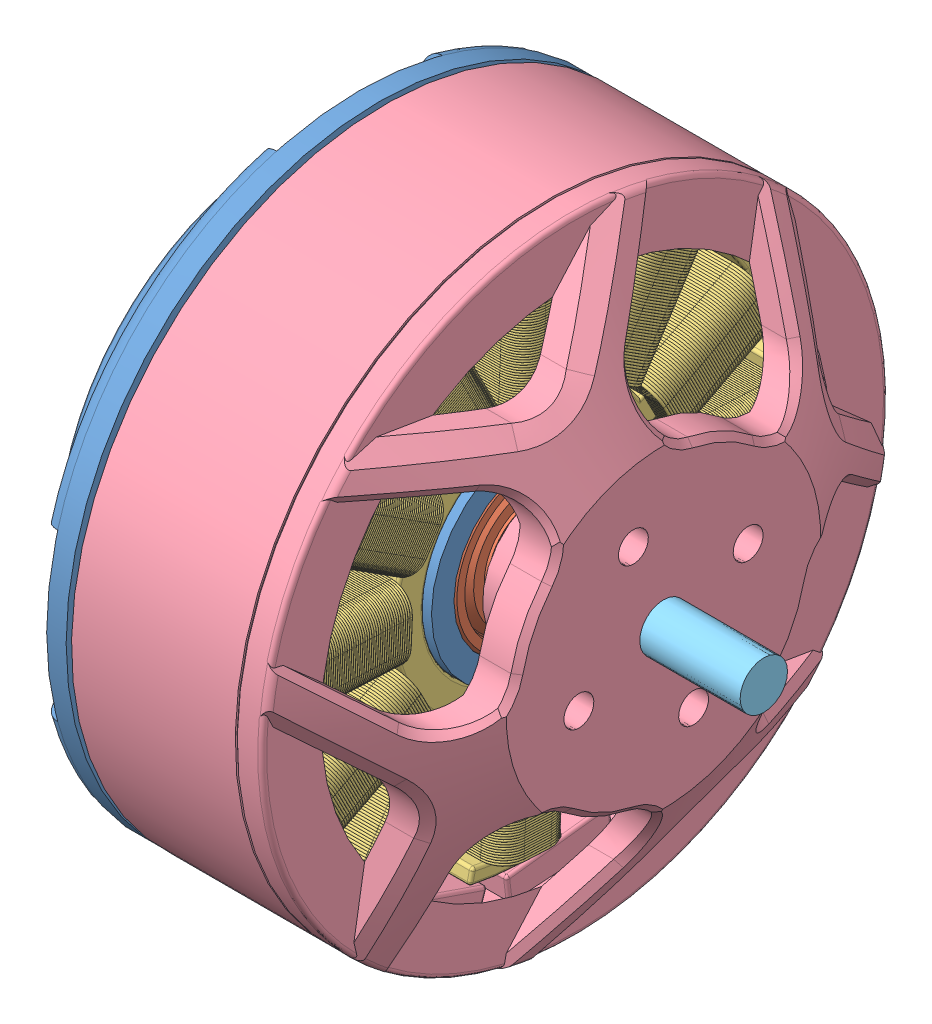
SolidWorks assembly 3508, configuration Default. Lengths in mm.
Overall size (33.2 53.4 53.4).
7 component instances, 6 part files, 12 mates.
Components (placement in the parent):
- stator-1: stator [Default] at origin size (17.19 41.8 41.8)
- R1140ZZ bearing-1: R1140ZZ bearing [Default] at (2 0 0) x (1 0 0) z (0 -0.171548 0.985176) size (4 11 11)
- R1140ZZ bearing-2: R1140ZZ bearing [Default] at (15 0 0) x (1 0 0) z (0 -0.050794 0.998709) size (4 11 11)
- coil_green-1: coil_green [Default] at (16.5 0 0) x (0 0.841823 -0.539754) z (0 0.539754 0.841823) size (36 10.71 36)
- bell-1: bell [Default] at (25.5 0 0) x (1 0 0) z (0 -0.335291 0.942115) size (18.64 41.8 41.8)
- axle-1: axle [Default] at (-1 0 0) x (0 -1 0) z (0 0 1) size (3.17 33.2 3.17)
- circlip-1: circlip [Default] x (0 1 0) z (0 0 1) size (4.2 0.2 3.63)
Mates (geometry in assembly coordinates):
- Concentric1: concentric: cylinder of stator-1 through (0 0 0) axis (1 0 0) radius 5.5; cylinder of R1140ZZ bearing-1 through (2 0 0) axis (-1 0 0) radius 1.585
- Coincident1: coincident: plane of stator-1 through (4 0 0) normal (-1 0 0); plane of R1140ZZ bearing-1 through (4 0 0) normal (1 0 0)
- Concentric2: concentric: cylinder of stator-1 through (0 0 0) axis (-1 0 0) radius 5.5; cylinder of R1140ZZ bearing-2 through (15 0 0) axis (-1 0 0) radius 5.5
- Coincident2: coincident: plane of stator-1 through (13 0 0) normal (1 0 0); plane of R1140ZZ bearing-2 through (13 0 0) normal (-1 0 0)
- Concentric3: concentric: cylinder of stator-1 through (0 0 0) axis (-1 0 0) radius 7; cylinder of coil_green-1 through (8.5 0 0) axis (1 0 0) radius 7
- Coincident3: coincident: plane of stator-1 through (8.5 0 0) normal (1 0 0); plane of coil_green-1 through (8.5 0 0) normal (-1 0 0)
- Concentric4: concentric: cylinder of stator-1 through (0 0 0) axis (-1 0 0) radius 2; cylinder of bell-1 through (23 0 0) axis (-1 0 0) radius 1.585
- Distance1: distance = 25.5 mm: plane of bell-1 through (25.5 1.4933 0.5314) normal (1 0 0); plane of stator-1 through (0 0 0) normal (-1 0 0)
- Concentric5: concentric: cylinder of bell-1 through (23 0 0) axis (-1 0 0) radius 1.585; cylinder of axle-1 through (32.2 0 0) axis (-1 0 0) radius 1.585
- Distance2: distance = 32.2 mm: plane of axle-1 through (32.2 0 0) normal (1 0 0); plane of stator-1 through (0 0 0) normal (-1 0 0)
- Concentric6: concentric: cylinder of axle-1 through (-2.7 0 0) axis (-1 0 0) radius 1.085; cylinder of circlip-1 through (-0.2 0 0) axis (1 0 0) radius 1.2
- Coincident6: coincident: plane of axle-1 through (0 0 0) normal (-1 0 0); plane of circlip-1 through (0 0 0) normal (1 0 0)
